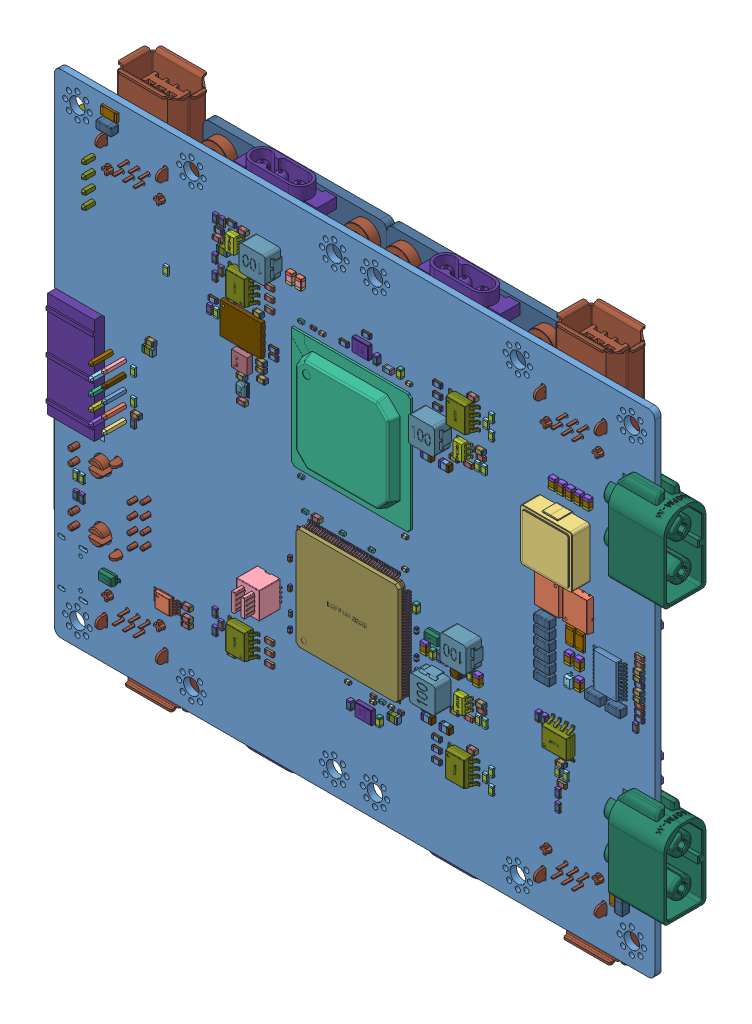
SolidWorks assembly Mother  Board, configuration 默认. Lengths in mm. (continued)
Components (placement in the parent): (continued)
- Mother  Board.step-1: Mother  Board.step [默认] at origin size (122.6 102.08 21) (continued)
  - Free-Models.step-1: Free-Models.step [默认] at origin size (70.87 98.07 8.62) (continued)
    - Driver_Board.step-3: Driver_Board.step [默认] at (57.3933 0 -6.2) x (1 0 0) z (0 0 1) size (35.43 49.03 8.62) (continued)
      - CP4-1.step-1: CP4-1.step [默认] at origin size (1.5 3 1.5)
        - (______)-94.step-1: (______)-94.step [默认] at (7.4932 17.145 0) x (1 0 0) z (0 0 1) size (1.5 3 1.5)
      - CP3-1.step-1: CP3-1.step [默认] at origin size (1.5 3 1.5)
        - (______)-94.step-1: (______)-94.step [默认] at (27.3051 17.1449 0) x (1 0 0) z (0 0 1) size (1.5 3 1.5)
      - CP2-1.step-1: CP2-1.step [默认] at origin size (1.5 3 1.5)
        - (______)-94.step-1: (______)-94.step [默认] at (16.3831 19.4309 0) x (1 0 0) z (0 0 1) size (1.5 3 1.5)
      - CP1-1.step-1: CP1-1.step [默认] at origin size (1.5 3 1.5)
        - (______)-94.step-1: (______)-94.step [默认] at (5.5882 17.145 0) x (1 0 0) z (0 0 1) size (1.5 3 1.5)
      - C29-1.step-1: C29-1.step [默认] at origin size (1.6 0.8 0.8)
        - 6547515616.step-1: 6547515616.step [默认] at (22.9869 16.6369 0) x (-1 0 0) z (0 0 1) size (1.6 0.8 0.8)
          - Terminal-22.step-1: Terminal-22.step [默认] at (-0.8 -0.4 0) size (1.6 0.8 0.8)
            - Open_CASCADE_STEP_translator_6.8_47.1.1-85.step-1: Open_CASCADE_STEP_translator_6.8_47.1.1-85.step [默认] at origin size (0.3 0.8 0.8)
            - Open_CASCADE_STEP_translator_6.8_47.1.2-86.step-1: Open_CASCADE_STEP_translator_6.8_47.1.2-86.step [默认] at origin size (0.3 0.8 0.8)
          - Mid_Body-10.step-1: Mid_Body-10.step [默认] at (-0.8 -0.4 0) size (1 0.8 0.8)
            - Open_CASCADE_STEP_translator_6.8_47.2.1-87.step-1: Open_CASCADE_STEP_translator_6.8_47.2.1-87.step [默认] at origin size (1 0.8 0.8)
      - C28-1.step-1: C28-1.step [默认] at origin size (1.6 0.8 0.8)
        - 6547515616.step-1: 6547515616.step [默认] at (24.6379 10.6679 0) x (-1 0 0) z (0 0 1) size (1.6 0.8 0.8)
          - Terminal-22.step-1: Terminal-22.step [默认] at (-0.8 -0.4 0) size (1.6 0.8 0.8)
            - Open_CASCADE_STEP_translator_6.8_47.1.1-85.step-1: Open_CASCADE_STEP_translator_6.8_47.1.1-85.step [默认] at origin size (0.3 0.8 0.8)
            - Open_CASCADE_STEP_translator_6.8_47.1.2-86.step-1: Open_CASCADE_STEP_translator_6.8_47.1.2-86.step [默认] at origin size (0.3 0.8 0.8)
          - Mid_Body-10.step-1: Mid_Body-10.step [默认] at (-0.8 -0.4 0) size (1 0.8 0.8)
            - Open_CASCADE_STEP_translator_6.8_47.2.1-87.step-1: Open_CASCADE_STEP_translator_6.8_47.2.1-87.step [默认] at origin size (1 0.8 0.8)
      - C27-1.step-1: C27-1.step [默认] at origin size (2.01 1.25 0.94)
        - 6547513136.step-1: 6547513136.step [默认] at (20.8503 23.4725 0) x (-1 0 0) z (0 0 1) size (2.01 1.25 0.94)
          - Fillet1-95.step-1: Fillet1-95.step [默认] at origin size (0.5 1.25 0.94)
          - Fillet2-96.step-1: Fillet2-96.step [默认] at origin size (0.5 1.25 0.94)
          - body2-97.step-1: body2-97.step [默认] at origin size (1.01 1.22 0.92)
      - C26-1.step-1: C26-1.step [默认] at origin size (0.8 1.6 0.8)
        - 6547516096.step-1: 6547516096.step [默认] at (17.9295 24.7425 0) x (0 -1 0) z (0 0 1) size (1.6 0.8 0.8)
          - Terminal-23.step-1: Terminal-23.step [默认] at (-0.8 -0.4 0) size (1.6 0.8 0.8)
            - Open_CASCADE_STEP_translator_6.8_47.1.1-98.step-1: Open_CASCADE_STEP_translator_6.8_47.1.1-98.step [默认] at origin size (0.3 0.8 0.8)
            - Open_CASCADE_STEP_translator_6.8_47.1.2-99.step-1: Open_CASCADE_STEP_translator_6.8_47.1.2-99.step [默认] at origin size (0.3 0.8 0.8)
          - Mid_Body-11.step-1: Mid_Body-11.step [默认] at (-0.8 -0.4 0) size (1 0.8 0.8)
            - Open_CASCADE_STEP_translator_6.8_47.2.1-100.step-1: Open_CASCADE_STEP_translator_6.8_47.2.1-100.step [默认] at origin size (1 0.8 0.8)
      - C25-1.step-1: C25-1.step [默认] at origin size (1.25 2.01 0.94)
        - 6547514896.step-1: 6547514896.step [默认] at (23.5173 31.0126 0) x (0 1 0) z (0 0 1) size (2.01 1.25 0.94)
          - Fillet1-101.step-1: Fillet1-101.step [默认] at origin size (0.5 1.25 0.94)
          - Fillet2-102.step-1: Fillet2-102.step [默认] at origin size (0.5 1.25 0.94)
          - body2-103.step-1: body2-103.step [默认] at origin size (1.01 1.22 0.92)
      - C20-1.step-1: C20-1.step [默认] at origin size (1.6 0.8 0.8)
        - 6547515616.step-1: 6547515616.step [默认] at (12.0649 18.9229 0) x (-1 0 0) z (0 0 1) size (1.6 0.8 0.8)
          - Terminal-22.step-1: Terminal-22.step [默认] at (-0.8 -0.4 0) size (1.6 0.8 0.8)
            - Open_CASCADE_STEP_translator_6.8_47.1.1-85.step-1: Open_CASCADE_STEP_translator_6.8_47.1.1-85.step [默认] at origin size (0.3 0.8 0.8)
            - Open_CASCADE_STEP_translator_6.8_47.1.2-86.step-1: Open_CASCADE_STEP_translator_6.8_47.1.2-86.step [默认] at origin size (0.3 0.8 0.8)
          - Mid_Body-10.step-1: Mid_Body-10.step [默认] at (-0.8 -0.4 0) size (1 0.8 0.8)
            - Open_CASCADE_STEP_translator_6.8_47.2.1-87.step-1: Open_CASCADE_STEP_translator_6.8_47.2.1-87.step [默认] at origin size (1 0.8 0.8)
      - C19-1.step-1: C19-1.step [默认] at origin size (0.8 1.6 0.8)
        - 6547517776.step-1: 6547517776.step [默认] at (25.7809 37.7191 0) x (0 1 0) z (0 0 1) size (1.6 0.8 0.8)
          - Terminal-24.step-1: Terminal-24.step [默认] at (-0.8 -0.4 0) size (1.6 0.8 0.8)
            - Open_CASCADE_STEP_translator_6.8_47.1.1-104.step-1: Open_CASCADE_STEP_translator_6.8_47.1.1-104.step [默认] at origin size (0.3 0.8 0.8)
            - Open_CASCADE_STEP_translator_6.8_47.1.2-105.step-1: Open_CASCADE_STEP_translator_6.8_47.1.2-105.step [默认] at origin size (0.3 0.8 0.8)
          - Mid_Body-12.step-1: Mid_Body-12.step [默认] at (-0.8 -0.4 0) size (1 0.8 0.8)
            - Open_CASCADE_STEP_translator_6.8_47.2.1-106.step-1: Open_CASCADE_STEP_translator_6.8_47.2.1-106.step [默认] at origin size (1 0.8 0.8)
      - C18-1.step-1: C18-1.step [默认] at origin size (0.8 1.6 0.8)
        - 6547517776.step-1: 6547517776.step [默认] at (24.6379 37.7191 0) x (0 1 0) z (0 0 1) size (1.6 0.8 0.8)
          - Terminal-24.step-1: Terminal-24.step [默认] at (-0.8 -0.4 0) size (1.6 0.8 0.8)
            - Open_CASCADE_STEP_translator_6.8_47.1.1-104.step-1: Open_CASCADE_STEP_translator_6.8_47.1.1-104.step [默认] at origin size (0.3 0.8 0.8)
            - Open_CASCADE_STEP_translator_6.8_47.1.2-105.step-1: Open_CASCADE_STEP_translator_6.8_47.1.2-105.step [默认] at origin size (0.3 0.8 0.8)
          - Mid_Body-12.step-1: Mid_Body-12.step [默认] at (-0.8 -0.4 0) size (1 0.8 0.8)
            - Open_CASCADE_STEP_translator_6.8_47.2.1-106.step-1: Open_CASCADE_STEP_translator_6.8_47.2.1-106.step [默认] at origin size (1 0.8 0.8)
      - C17-1.step-1: C17-1.step [默认] at origin size (1.6 0.8 0.8)
        - 6547515616.step-1: 6547515616.step [默认] at (13.7159 12.9539 0) x (-1 0 0) z (0 0 1) size (1.6 0.8 0.8)
          - Terminal-22.step-1: Terminal-22.step [默认] at (-0.8 -0.4 0) size (1.6 0.8 0.8)
            - Open_CASCADE_STEP_translator_6.8_47.1.1-85.step-1: Open_CASCADE_STEP_translator_6.8_47.1.1-85.step [默认] at origin size (0.3 0.8 0.8)
            - Open_CASCADE_STEP_translator_6.8_47.1.2-86.step-1: Open_CASCADE_STEP_translator_6.8_47.1.2-86.step [默认] at origin size (0.3 0.8 0.8)
          - Mid_Body-10.step-1: Mid_Body-10.step [默认] at (-0.8 -0.4 0) size (1 0.8 0.8)
            - Open_CASCADE_STEP_translator_6.8_47.2.1-87.step-1: Open_CASCADE_STEP_translator_6.8_47.2.1-87.step [默认] at origin size (1 0.8 0.8)
      - C16-1.step-1: C16-1.step [默认] at origin size (0.8 1.6 0.8)
        - 6547516096.step-1: 6547516096.step [默认] at (25.7811 22.2249 0) x (0 -1 0) z (0 0 1) size (1.6 0.8 0.8)
          - Terminal-23.step-1: Terminal-23.step [默认] at (-0.8 -0.4 0) size (1.6 0.8 0.8)
            - Open_CASCADE_STEP_translator_6.8_47.1.1-98.step-1: Open_CASCADE_STEP_translator_6.8_47.1.1-98.step [默认] at origin size (0.3 0.8 0.8)
            - Open_CASCADE_STEP_translator_6.8_47.1.2-99.step-1: Open_CASCADE_STEP_translator_6.8_47.1.2-99.step [默认] at origin size (0.3 0.8 0.8)
          - Mid_Body-11.step-1: Mid_Body-11.step [默认] at (-0.8 -0.4 0) size (1 0.8 0.8)
            - Open_CASCADE_STEP_translator_6.8_47.2.1-100.step-1: Open_CASCADE_STEP_translator_6.8_47.2.1-100.step [默认] at origin size (1 0.8 0.8)
      - C15-1.step-1: C15-1.step [默认] at origin size (0.8 1.6 0.8)
        - 6547517776.step-1: 6547517776.step [默认] at (23.8759 25.6541 0) x (0 1 0) z (0 0 1) size (1.6 0.8 0.8)
          - Terminal-24.step-1: Terminal-24.step [默认] at (-0.8 -0.4 0) size (1.6 0.8 0.8)
            - Open_CASCADE_STEP_translator_6.8_47.1.1-104.step-1: Open_CASCADE_STEP_translator_6.8_47.1.1-104.step [默认] at origin size (0.3 0.8 0.8)
            - Open_CASCADE_STEP_translator_6.8_47.1.2-105.step-1: Open_CASCADE_STEP_translator_6.8_47.1.2-105.step [默认] at origin size (0.3 0.8 0.8)
          - Mid_Body-12.step-1: Mid_Body-12.step [默认] at (-0.8 -0.4 0) size (1 0.8 0.8)
            - Open_CASCADE_STEP_translator_6.8_47.2.1-106.step-1: Open_CASCADE_STEP_translator_6.8_47.2.1-106.step [默认] at origin size (1 0.8 0.8)
      - C14-1.step-1: C14-1.step [默认] at origin size (2.01 1.25 0.94)
        - 6547513136.step-1: 6547513136.step [默认] at (13.7383 23.4725 0) x (-1 0 0) z (0 0 1) size (2.01 1.25 0.94)
          - Fillet1-95.step-1: Fillet1-95.step [默认] at origin size (0.5 1.25 0.94)
          - Fillet2-96.step-1: Fillet2-96.step [默认] at origin size (0.5 1.25 0.94)
          - body2-97.step-1: body2-97.step [默认] at origin size (1.01 1.22 0.92)
      - C13-1.step-1: C13-1.step [默认] at origin size (0.8 1.6 0.8)
        - 6547516096.step-1: 6547516096.step [默认] at (10.8175 24.7425 0) x (0 -1 0) z (0 0 1) size (1.6 0.8 0.8)
          - Terminal-23.step-1: Terminal-23.step [默认] at (-0.8 -0.4 0) size (1.6 0.8 0.8)
            - Open_CASCADE_STEP_translator_6.8_47.1.1-98.step-1: Open_CASCADE_STEP_translator_6.8_47.1.1-98.step [默认] at origin size (0.3 0.8 0.8)
            - Open_CASCADE_STEP_translator_6.8_47.1.2-99.step-1: Open_CASCADE_STEP_translator_6.8_47.1.2-99.step [默认] at origin size (0.3 0.8 0.8)
          - Mid_Body-11.step-1: Mid_Body-11.step [默认] at (-0.8 -0.4 0) size (1 0.8 0.8)
            - Open_CASCADE_STEP_translator_6.8_47.2.1-100.step-1: Open_CASCADE_STEP_translator_6.8_47.2.1-100.step [默认] at origin size (1 0.8 0.8)
      - C12-1.step-1: C12-1.step [默认] at origin size (1.25 2.01 0.94)
        - 6547514896.step-1: 6547514896.step [默认] at (16.4053 31.0126 0) x (0 1 0) z (0 0 1) size (2.01 1.25 0.94)
          - Fillet1-101.step-1: Fillet1-101.step [默认] at origin size (0.5 1.25 0.94)
          - Fillet2-102.step-1: Fillet2-102.step [默认] at origin size (0.5 1.25 0.94)
          - body2-103.step-1: body2-103.step [默认] at origin size (1.01 1.22 0.92)
      - C11-1.step-1: C11-1.step [默认] at origin size (1.6 0.8 0.8)
        - 6547515616.step-1: 6547515616.step [默认] at (27.6859 22.8599 0) x (-1 0 0) z (0 0 1) size (1.6 0.8 0.8)
          - Terminal-22.step-1: Terminal-22.step [默认] at (-0.8 -0.4 0) size (1.6 0.8 0.8)
            - Open_CASCADE_STEP_translator_6.8_47.1.1-85.step-1: Open_CASCADE_STEP_translator_6.8_47.1.1-85.step [默认] at origin size (0.3 0.8 0.8)
            - Open_CASCADE_STEP_translator_6.8_47.1.2-86.step-1: Open_CASCADE_STEP_translator_6.8_47.1.2-86.step [默认] at origin size (0.3 0.8 0.8)
          - Mid_Body-10.step-1: Mid_Body-10.step [默认] at (-0.8 -0.4 0) size (1 0.8 0.8)
            - Open_CASCADE_STEP_translator_6.8_47.2.1-87.step-1: Open_CASCADE_STEP_translator_6.8_47.2.1-87.step [默认] at origin size (1 0.8 0.8)
      - C10-1.step-1: C10-1.step [默认] at origin size (0.8 1.6 0.8)
        - 6547517776.step-1: 6547517776.step [默认] at (-3.1751 37.7191 0) x (0 1 0) z (0 0 1) size (1.6 0.8 0.8)
          - Terminal-24.step-1: Terminal-24.step [默认] at (-0.8 -0.4 0) size (1.6 0.8 0.8)
            - Open_CASCADE_STEP_translator_6.8_47.1.1-104.step-1: Open_CASCADE_STEP_translator_6.8_47.1.1-104.step [默认] at origin size (0.3 0.8 0.8)
            - Open_CASCADE_STEP_translator_6.8_47.1.2-105.step-1: Open_CASCADE_STEP_translator_6.8_47.1.2-105.step [默认] at origin size (0.3 0.8 0.8)
          - Mid_Body-12.step-1: Mid_Body-12.step [默认] at (-0.8 -0.4 0) size (1 0.8 0.8)
            - Open_CASCADE_STEP_translator_6.8_47.2.1-106.step-1: Open_CASCADE_STEP_translator_6.8_47.2.1-106.step [默认] at origin size (1 0.8 0.8)
      - C9-1.step-1: C9-1.step [默认] at origin size (0.8 1.6 0.8)
        - 6547516096.step-1: 6547516096.step [默认] at (-3.1749 22.2249 0) x (0 -1 0) z (0 0 1) size (1.6 0.8 0.8)
          - Terminal-23.step-1: Terminal-23.step [默认] at (-0.8 -0.4 0) size (1.6 0.8 0.8)
            - Open_CASCADE_STEP_translator_6.8_47.1.1-98.step-1: Open_CASCADE_STEP_translator_6.8_47.1.1-98.step [默认] at origin size (0.3 0.8 0.8)
            - Open_CASCADE_STEP_translator_6.8_47.1.2-99.step-1: Open_CASCADE_STEP_translator_6.8_47.1.2-99.step [默认] at origin size (0.3 0.8 0.8)
          - Mid_Body-11.step-1: Mid_Body-11.step [默认] at (-0.8 -0.4 0) size (1 0.8 0.8)
            - Open_CASCADE_STEP_translator_6.8_47.2.1-100.step-1: Open_CASCADE_STEP_translator_6.8_47.2.1-100.step [默认] at origin size (1 0.8 0.8)
      - C8-1.step-1: C8-1.step [默认] at origin size (1.6 0.8 0.8)
        - 6547515616.step-1: 6547515616.step [默认] at (1.1429 16.5099 0) x (-1 0 0) z (0 0 1) size (1.6 0.8 0.8)
          - Terminal-22.step-1: Terminal-22.step [默认] at (-0.8 -0.4 0) size (1.6 0.8 0.8)
            - Open_CASCADE_STEP_translator_6.8_47.1.1-85.step-1: Open_CASCADE_STEP_translator_6.8_47.1.1-85.step [默认] at origin size (0.3 0.8 0.8)
            - Open_CASCADE_STEP_translator_6.8_47.1.2-86.step-1: Open_CASCADE_STEP_translator_6.8_47.1.2-86.step [默认] at origin size (0.3 0.8 0.8)
          - Mid_Body-10.step-1: Mid_Body-10.step [默认] at (-0.8 -0.4 0) size (1 0.8 0.8)
            - Open_CASCADE_STEP_translator_6.8_47.2.1-87.step-1: Open_CASCADE_STEP_translator_6.8_47.2.1-87.step [默认] at origin size (1 0.8 0.8)
      - C7-1.step-1: C7-1.step [默认] at origin size (0.8 1.6 0.8)
        - 6547516096.step-1: 6547516096.step [默认] at (-2.0319 22.2249 0) x (0 -1 0) z (0 0 1) size (1.6 0.8 0.8)
          - Terminal-23.step-1: Terminal-23.step [默认] at (-0.8 -0.4 0) size (1.6 0.8 0.8)
            - Open_CASCADE_STEP_translator_6.8_47.1.1-98.step-1: Open_CASCADE_STEP_translator_6.8_47.1.1-98.step [默认] at origin size (0.3 0.8 0.8)
            - Open_CASCADE_STEP_translator_6.8_47.1.2-99.step-1: Open_CASCADE_STEP_translator_6.8_47.1.2-99.step [默认] at origin size (0.3 0.8 0.8)
          - Mid_Body-11.step-1: Mid_Body-11.step [默认] at (-0.8 -0.4 0) size (1 0.8 0.8)
            - Open_CASCADE_STEP_translator_6.8_47.2.1-100.step-1: Open_CASCADE_STEP_translator_6.8_47.2.1-100.step [默认] at origin size (1 0.8 0.8)
      - C6-1.step-1: C6-1.step [默认] at origin size (0.8 1.6 0.8)
        - 6547517776.step-1: 6547517776.step [默认] at (-2.0321 37.7191 0) x (0 1 0) z (0 0 1) size (1.6 0.8 0.8)
          - Terminal-24.step-1: Terminal-24.step [默认] at (-0.8 -0.4 0) size (1.6 0.8 0.8)
            - Open_CASCADE_STEP_translator_6.8_47.1.1-104.step-1: Open_CASCADE_STEP_translator_6.8_47.1.1-104.step [默认] at origin size (0.3 0.8 0.8)
            - Open_CASCADE_STEP_translator_6.8_47.1.2-105.step-1: Open_CASCADE_STEP_translator_6.8_47.1.2-105.step [默认] at origin size (0.3 0.8 0.8)
          - Mid_Body-12.step-1: Mid_Body-12.step [默认] at (-0.8 -0.4 0) size (1 0.8 0.8)
            - Open_CASCADE_STEP_translator_6.8_47.2.1-106.step-1: Open_CASCADE_STEP_translator_6.8_47.2.1-106.step [默认] at origin size (1 0.8 0.8)
      - C5-1.step-1: C5-1.step [默认] at origin size (1.6 0.8 0.8)
        - 6547515616.step-1: 6547515616.step [默认] at (2.7939 10.6679 0) x (-1 0 0) z (0 0 1) size (1.6 0.8 0.8)
          - Terminal-22.step-1: Terminal-22.step [默认] at (-0.8 -0.4 0) size (1.6 0.8 0.8)
            - Open_CASCADE_STEP_translator_6.8_47.1.1-85.step-1: Open_CASCADE_STEP_translator_6.8_47.1.1-85.step [默认] at origin size (0.3 0.8 0.8)
            - Open_CASCADE_STEP_translator_6.8_47.1.2-86.step-1: Open_CASCADE_STEP_translator_6.8_47.1.2-86.step [默认] at origin size (0.3 0.8 0.8)
          - Mid_Body-10.step-1: Mid_Body-10.step [默认] at (-0.8 -0.4 0) size (1 0.8 0.8)
            - Open_CASCADE_STEP_translator_6.8_47.2.1-87.step-1: Open_CASCADE_STEP_translator_6.8_47.2.1-87.step [默认] at origin size (1 0.8 0.8)
      - C4-1.step-1: C4-1.step [默认] at origin size (1.6 0.8 0.8)
        - 6547515616.step-1: 6547515616.step [默认] at (-0.1271 22.8599 0) x (-1 0 0) z (0 0 1) size (1.6 0.8 0.8)
          - Terminal-22.step-1: Terminal-22.step [默认] at (-0.8 -0.4 0) size (1.6 0.8 0.8)
            - Open_CASCADE_STEP_translator_6.8_47.1.1-85.step-1: Open_CASCADE_STEP_translator_6.8_47.1.1-85.step [默认] at origin size (0.3 0.8 0.8)
            - Open_CASCADE_STEP_translator_6.8_47.1.2-86.step-1: Open_CASCADE_STEP_translator_6.8_47.1.2-86.step [默认] at origin size (0.3 0.8 0.8)
          - Mid_Body-10.step-1: Mid_Body-10.step [默认] at (-0.8 -0.4 0) size (1 0.8 0.8)
            - Open_CASCADE_STEP_translator_6.8_47.2.1-87.step-1: Open_CASCADE_STEP_translator_6.8_47.2.1-87.step [默认] at origin size (1 0.8 0.8)
      - C3-1.step-1: C3-1.step [默认] at origin size (2.01 1.25 0.94)
        - 6547513136.step-1: 6547513136.step [默认] at (6.6263 23.4725 0) x (-1 0 0) z (0 0 1) size (2.01 1.25 0.94)
          - Fillet1-95.step-1: Fillet1-95.step [默认] at origin size (0.5 1.25 0.94)
          - Fillet2-96.step-1: Fillet2-96.step [默认] at origin size (0.5 1.25 0.94)
          - body2-97.step-1: body2-97.step [默认] at origin size (1.01 1.22 0.92)
      - C2-1.step-1: C2-1.step [默认] at origin size (0.8 1.6 0.8)
        - 6547516096.step-1: 6547516096.step [默认] at (3.7055 24.7425 0) x (0 -1 0) z (0 0 1) size (1.6 0.8 0.8)
          - Terminal-23.step-1: Terminal-23.step [默认] at (-0.8 -0.4 0) size (1.6 0.8 0.8)
            - Open_CASCADE_STEP_translator_6.8_47.1.1-98.step-1: Open_CASCADE_STEP_translator_6.8_47.1.1-98.step [默认] at origin size (0.3 0.8 0.8)
            - Open_CASCADE_STEP_translator_6.8_47.1.2-99.step-1: Open_CASCADE_STEP_translator_6.8_47.1.2-99.step [默认] at origin size (0.3 0.8 0.8)
          - Mid_Body-11.step-1: Mid_Body-11.step [默认] at (-0.8 -0.4 0) size (1 0.8 0.8)
            - Open_CASCADE_STEP_translator_6.8_47.2.1-100.step-1: Open_CASCADE_STEP_translator_6.8_47.2.1-100.step [默认] at origin size (1 0.8 0.8)
      - C1.step-1: C1.step [默认] at origin size (1.25 2.01 0.94)
        - 6547514896.step-1: 6547514896.step [默认] at (9.2933 31.0126 0) x (0 1 0) z (0 0 1) size (2.01 1.25 0.94)
          - Fillet1-101.step-1: Fillet1-101.step [默认] at origin size (0.5 1.25 0.94)
          - Fillet2-102.step-1: Fillet2-102.step [默认] at origin size (0.5 1.25 0.94)
          - body2-103.step-1: body2-103.step [默认] at origin size (1.01 1.22 0.92)
    - Driver_Board.step-4: Driver_Board.step [默认] at (21.971 0 -6.2) x (1 0 0) z (0 0 1) size (35.43 49.03 8.62)
      - Board-1.step-1: Board-1.step [默认] at origin size (35.43 46.99 1.62)
        - Open_CASCADE_STEP_translator_6.8_2.1.1.step-1: Open_CASCADE_STEP_translator_6.8_2.1.1.step [默认] at (0 0 -1.6164) size (35.43 46.99 1.62)
      - R25-1.step-1: R25-1.step [默认] at origin size (0.8 1.6 0.45)
        - 6547515376.step-1: 6547515376.step [默认] at (20.6304 35.5601 0) x (0 1 0) z (0 0 1) size (1.6 0.8 0.45)
          - Terminal-19.step-1: Terminal-19.step [默认] at (-0.8 -0.4 0) size (0.3 0.8 0.45)
            - Open_CASCADE_STEP_translator_6.8_21.2.1-76.step-1: Open_CASCADE_STEP_translator_6.8_21.2.1-76.step [默认] at origin size (0.3 0.8 0.45)
          - Terminal-19.step-2: Terminal-19.step [默认] at (0.8 0.4 0) x (-1 0 0) z (0 0 1) size (0.3 0.8 0.45)
            - Open_CASCADE_STEP_translator_6.8_21.2.1-76.step-1: Open_CASCADE_STEP_translator_6.8_21.2.1-76.step [默认] at origin size (0.3 0.8 0.45)
          - Mid_Body-77.step-1: Mid_Body-77.step [默认] at (-0.8 -0.4 0) size (1.51 0.8 0.36)
          - Mark-78.step-1: Mark-78.step [默认] at (-0.5 -0.4 0.405) size (1 0.8 0.05)
      - R24-1.step-1: R24-1.step [默认] at origin size (1.6 0.8 0.45)
        - 6547516336.step-1: 6547516336.step [默认] at (12.6999 34.9249 0) x (-1 0 0) z (0 0 1) size (1.6 0.8 0.45)
          - Terminal-20.step-1: Terminal-20.step [默认] at (-0.8 -0.4 0) size (0.3 0.8 0.45)
            - Open_CASCADE_STEP_translator_6.8_21.2.1-79.step-1: Open_CASCADE_STEP_translator_6.8_21.2.1-79.step [默认] at origin size (0.3 0.8 0.45)
          - Terminal-20.step-2: Terminal-20.step [默认] at (0.8 0.4 0) x (-1 0 0) z (0 0 1) size (0.3 0.8 0.45)
            - Open_CASCADE_STEP_translator_6.8_21.2.1-79.step-1: Open_CASCADE_STEP_translator_6.8_21.2.1-79.step [默认] at origin size (0.3 0.8 0.45)
          - Mid_Body-80.step-1: Mid_Body-80.step [默认] at (-0.8 -0.4 0) size (1.51 0.8 0.36)
          - Mark-81.step-1: Mark-81.step [默认] at (-0.5 -0.4 0.405) size (1 0.8 0.05)
      - R23-1.step-1: R23-1.step [默认] at origin size (1.6 0.8 0.45)
        - 6547516336.step-1: 6547516336.step [默认] at (5.5879 33.6549 0) x (-1 0 0) z (0 0 1) size (1.6 0.8 0.45)
          - Terminal-20.step-1: Terminal-20.step [默认] at (-0.8 -0.4 0) size (0.3 0.8 0.45)
            - Open_CASCADE_STEP_translator_6.8_21.2.1-79.step-1: Open_CASCADE_STEP_translator_6.8_21.2.1-79.step [默认] at origin size (0.3 0.8 0.45)
          - Terminal-20.step-2: Terminal-20.step [默认] at (0.8 0.4 0) x (-1 0 0) z (0 0 1) size (0.3 0.8 0.45)
            - Open_CASCADE_STEP_translator_6.8_21.2.1-79.step-1: Open_CASCADE_STEP_translator_6.8_21.2.1-79.step [默认] at origin size (0.3 0.8 0.45)
          - Mid_Body-80.step-1: Mid_Body-80.step [默认] at (-0.8 -0.4 0) size (1.51 0.8 0.36)
          - Mark-81.step-1: Mark-81.step [默认] at (-0.5 -0.4 0.405) size (1 0.8 0.05)
      - JP1.step-1: JP1.step [默认] at origin size (16.01 14.49 6.96)
        - User_Library-MR30PW-M.step-1: User_Library-MR30PW-M.step [默认] at (13.7158 -5.9802 2.75) x (1 0 0) z (0 0 1) size (16.01 14.49 6.96)
      - R18-1.step-1: R18-1.step [默认] at origin size (0.8 1.6 0.45)
        - 6547515376.step-1: 6547515376.step [默认] at (22.9869 34.4171 0) x (0 1 0) z (0 0 1) size (1.6 0.8 0.45)
          - Terminal-19.step-1: Terminal-19.step [默认] at (-0.8 -0.4 0) size (0.3 0.8 0.45)
            - Open_CASCADE_STEP_translator_6.8_21.2.1-76.step-1: Open_CASCADE_STEP_translator_6.8_21.2.1-76.step [默认] at origin size (0.3 0.8 0.45)
          - Terminal-19.step-2: Terminal-19.step [默认] at (0.8 0.4 0) x (-1 0 0) z (0 0 1) size (0.3 0.8 0.45)
            - Open_CASCADE_STEP_translator_6.8_21.2.1-76.step-1: Open_CASCADE_STEP_translator_6.8_21.2.1-76.step [默认] at origin size (0.3 0.8 0.45)
          - Mid_Body-77.step-1: Mid_Body-77.step [默认] at (-0.8 -0.4 0) size (1.51 0.8 0.36)
          - Mark-78.step-1: Mark-78.step [默认] at (-0.5 -0.4 0.405) size (1 0.8 0.05)
      - R17-1.step-1: R17-1.step [默认] at origin size (0.8 1.6 0.45)
        - 6547515376.step-1: 6547515376.step [默认] at (21.8663 34.3947 0) x (0 1 0) z (0 0 1) size (1.6 0.8 0.45)
          - Terminal-19.step-1: Terminal-19.step [默认] at (-0.8 -0.4 0) size (0.3 0.8 0.45)
            - Open_CASCADE_STEP_translator_6.8_21.2.1-76.step-1: Open_CASCADE_STEP_translator_6.8_21.2.1-76.step [默认] at origin size (0.3 0.8 0.45)
          - Terminal-19.step-2: Terminal-19.step [默认] at (0.8 0.4 0) x (-1 0 0) z (0 0 1) size (0.3 0.8 0.45)
            - Open_CASCADE_STEP_translator_6.8_21.2.1-76.step-1: Open_CASCADE_STEP_translator_6.8_21.2.1-76.step [默认] at origin size (0.3 0.8 0.45)
          - Mid_Body-77.step-1: Mid_Body-77.step [默认] at (-0.8 -0.4 0) size (1.51 0.8 0.36)
          - Mark-78.step-1: Mark-78.step [默认] at (-0.5 -0.4 0.405) size (1 0.8 0.05)
      - R16-1.step-1: R16-1.step [默认] at origin size (1.6 0.8 0.45)
        - 6547506496.step-1: 6547506496.step [默认] at (16.6371 33.6551 0) x (1 0 0) z (0 0 1) size (1.6 0.8 0.45)
          - Terminal-21.step-1: Terminal-21.step [默认] at (-0.8 -0.4 0) size (0.3 0.8 0.45)
            - Open_CASCADE_STEP_translator_6.8_21.2.1-82.step-1: Open_CASCADE_STEP_translator_6.8_21.2.1-82.step [默认] at origin size (0.3 0.8 0.45)
          - Terminal-21.step-2: Terminal-21.step [默认] at (0.8 0.4 0) x (-1 0 0) z (0 0 1) size (0.3 0.8 0.45)
            - Open_CASCADE_STEP_translator_6.8_21.2.1-82.step-1: Open_CASCADE_STEP_translator_6.8_21.2.1-82.step [默认] at origin size (0.3 0.8 0.45)
          - Mid_Body-83.step-1: Mid_Body-83.step [默认] at (-0.8 -0.4 0) size (1.51 0.8 0.36)
          - Mark-84.step-1: Mark-84.step [默认] at (-0.5 -0.4 0.405) size (1 0.8 0.05)
      - R15-1.step-1: R15-1.step [默认] at origin size (0.8 1.6 0.45)
        - 6547515376.step-1: 6547515376.step [默认] at (14.7319 34.2901 0) x (0 1 0) z (0 0 1) size (1.6 0.8 0.45)
          - Terminal-19.step-1: Terminal-19.step [默认] at (-0.8 -0.4 0) size (0.3 0.8 0.45)
            - Open_CASCADE_STEP_translator_6.8_21.2.1-76.step-1: Open_CASCADE_STEP_translator_6.8_21.2.1-76.step [默认] at origin size (0.3 0.8 0.45)
          - Terminal-19.step-2: Terminal-19.step [默认] at (0.8 0.4 0) x (-1 0 0) z (0 0 1) size (0.3 0.8 0.45)
            - Open_CASCADE_STEP_translator_6.8_21.2.1-76.step-1: Open_CASCADE_STEP_translator_6.8_21.2.1-76.step [默认] at origin size (0.3 0.8 0.45)
          - Mid_Body-77.step-1: Mid_Body-77.step [默认] at (-0.8 -0.4 0) size (1.51 0.8 0.36)
          - Mark-78.step-1: Mark-78.step [默认] at (-0.5 -0.4 0.405) size (1 0.8 0.05)
      - R13-1.step-1: R13-1.step [默认] at origin size (1.6 0.8 0.45)
        - 6547506496.step-1: 6547506496.step [默认] at (9.5251 33.6551 0) x (1 0 0) z (0 0 1) size (1.6 0.8 0.45)
          - Terminal-21.step-1: Terminal-21.step [默认] at (-0.8 -0.4 0) size (0.3 0.8 0.45)
            - Open_CASCADE_STEP_translator_6.8_21.2.1-82.step-1: Open_CASCADE_STEP_translator_6.8_21.2.1-82.step [默认] at origin size (0.3 0.8 0.45)
          - Terminal-21.step-2: Terminal-21.step [默认] at (0.8 0.4 0) x (-1 0 0) z (0 0 1) size (0.3 0.8 0.45)
            - Open_CASCADE_STEP_translator_6.8_21.2.1-82.step-1: Open_CASCADE_STEP_translator_6.8_21.2.1-82.step [默认] at origin size (0.3 0.8 0.45)
          - Mid_Body-83.step-1: Mid_Body-83.step [默认] at (-0.8 -0.4 0) size (1.51 0.8 0.36)
          - Mark-84.step-1: Mark-84.step [默认] at (-0.5 -0.4 0.405) size (1 0.8 0.05)
      - R11-1.step-1: R11-1.step [默认] at origin size (0.8 1.6 0.45)
        - 6547515376.step-1: 6547515376.step [默认] at (7.6423 34.2901 0) x (0 1 0) z (0 0 1) size (1.6 0.8 0.45)
          - Terminal-19.step-1: Terminal-19.step [默认] at (-0.8 -0.4 0) size (0.3 0.8 0.45)
            - Open_CASCADE_STEP_translator_6.8_21.2.1-76.step-1: Open_CASCADE_STEP_translator_6.8_21.2.1-76.step [默认] at origin size (0.3 0.8 0.45)
          - Terminal-19.step-2: Terminal-19.step [默认] at (0.8 0.4 0) x (-1 0 0) z (0 0 1) size (0.3 0.8 0.45)
            - Open_CASCADE_STEP_translator_6.8_21.2.1-76.step-1: Open_CASCADE_STEP_translator_6.8_21.2.1-76.step [默认] at origin size (0.3 0.8 0.45)
          - Mid_Body-77.step-1: Mid_Body-77.step [默认] at (-0.8 -0.4 0) size (1.51 0.8 0.36)
          - Mark-78.step-1: Mark-78.step [默认] at (-0.5 -0.4 0.405) size (1 0.8 0.05)
      - C23-1.step-1: C23-1.step [默认] at origin size (1.6 0.8 0.8)
        - 6547515616.step-1: 6547515616.step [默认] at (19.8684 33.6676 0) x (-1 0 0) z (0 0 1) size (1.6 0.8 0.8)
          - Terminal-22.step-1: Terminal-22.step [默认] at (-0.8 -0.4 0) size (1.6 0.8 0.8)
            - Open_CASCADE_STEP_translator_6.8_47.1.1-85.step-1: Open_CASCADE_STEP_translator_6.8_47.1.1-85.step [默认] at origin size (0.3 0.8 0.8)
            - Open_CASCADE_STEP_translator_6.8_47.1.2-86.step-1: Open_CASCADE_STEP_translator_6.8_47.1.2-86.step [默认] at origin size (0.3 0.8 0.8)
          - Mid_Body-10.step-1: Mid_Body-10.step [默认] at (-0.8 -0.4 0) size (1 0.8 0.8)
            - Open_CASCADE_STEP_translator_6.8_47.2.1-87.step-1: Open_CASCADE_STEP_translator_6.8_47.2.1-87.step [默认] at origin size (1 0.8 0.8)
      - C22-1.step-1: C22-1.step [默认] at origin size (1.6 0.8 0.8)
        - 6547515616.step-1: 6547515616.step [默认] at (12.6999 33.6549 0) x (-1 0 0) z (0 0 1) size (1.6 0.8 0.8)
          - Terminal-22.step-1: Terminal-22.step [默认] at (-0.8 -0.4 0) size (1.6 0.8 0.8)
            - Open_CASCADE_STEP_translator_6.8_47.1.1-85.step-1: Open_CASCADE_STEP_translator_6.8_47.1.1-85.step [默认] at origin size (0.3 0.8 0.8)
            - Open_CASCADE_STEP_translator_6.8_47.1.2-86.step-1: Open_CASCADE_STEP_translator_6.8_47.1.2-86.step [默认] at origin size (0.3 0.8 0.8)
          - Mid_Body-10.step-1: Mid_Body-10.step [默认] at (-0.8 -0.4 0) size (1 0.8 0.8)
            - Open_CASCADE_STEP_translator_6.8_47.2.1-87.step-1: Open_CASCADE_STEP_translator_6.8_47.2.1-87.step [默认] at origin size (1 0.8 0.8)
      - C21-1.step-1: C21-1.step [默认] at origin size (1.6 0.8 0.8)
        - 6547515616.step-1: 6547515616.step [默认] at (5.6103 34.9025 0) x (-1 0 0) z (0 0 1) size (1.6 0.8 0.8)
          - Terminal-22.step-1: Terminal-22.step [默认] at (-0.8 -0.4 0) size (1.6 0.8 0.8)
            - Open_CASCADE_STEP_translator_6.8_47.1.1-85.step-1: Open_CASCADE_STEP_translator_6.8_47.1.1-85.step [默认] at origin size (0.3 0.8 0.8)
            - Open_CASCADE_STEP_translator_6.8_47.1.2-86.step-1: Open_CASCADE_STEP_translator_6.8_47.1.2-86.step [默认] at origin size (0.3 0.8 0.8)
          - Mid_Body-10.step-1: Mid_Body-10.step [默认] at (-0.8 -0.4 0) size (1 0.8 0.8)
            - Open_CASCADE_STEP_translator_6.8_47.2.1-87.step-1: Open_CASCADE_STEP_translator_6.8_47.2.1-87.step [默认] at origin size (1 0.8 0.8)
      - U5-1.step-1: U5-1.step [默认] at origin size (5.9 11.5 2.7)
        - SO8_W.step-1: SO8_W.step [默认] at (27.6859 29.9721 0.381) x (0 1 0) z (0 0 1) size (11.5 5.9 2.7)
      - U4-1.step-1: U4-1.step [默认] at origin size (5.9 11.5 2.7)
        - SO8_W.step-1: SO8_W.step [默认] at (-0.1271 29.9721 0.381) x (0 1 0) z (0 0 1) size (11.5 5.9 2.7)
      - U3-1.step-1: U3-1.step [默认] at origin size (5 6.01 1.9)
        - SOP8-1.step-1: SOP8-1.step [默认] at (19.9615 29.5285 0) x (0 -1 0) z (0 0 1) size (6.01 5 1.9)
          - LOGO_-88.step-1: LOGO_-88.step [默认] at (0.0116 0 0.095) x (0 -1 0) z (0 0 -1) size (1.5 1.73 0.01)
          - SOP8-89.step-1: SOP8-89.step [默认] at origin size (6.01 5 1.9)
      - U2-1.step-1: U2-1.step [默认] at origin size (5 6.01 1.9)
        - SOP8-1.step-1: SOP8-1.step [默认] at (12.8495 29.5285 0) x (0 -1 0) z (0 0 1) size (6.01 5 1.9)
          - LOGO_-88.step-1: LOGO_-88.step [默认] at (0.0116 0 0.095) x (0 -1 0) z (0 0 -1) size (1.5 1.73 0.01)
          - SOP8-89.step-1: SOP8-89.step [默认] at origin size (6.01 5 1.9)
      - U1.step-1: U1.step [默认] at origin size (5 6.01 1.9)
        - SOP8-1.step-1: SOP8-1.step [默认] at (5.7375 29.5285 0) x (0 -1 0) z (0 0 1) size (6.01 5 1.9)
          - LOGO_-88.step-1: LOGO_-88.step [默认] at (0.0116 0 0.095) x (0 -1 0) z (0 0 -1) size (1.5 1.73 0.01)
          - SOP8-89.step-1: SOP8-89.step [默认] at origin size (6.01 5 1.9)
      - RS2-1.step-1: RS2-1.step [默认] at origin size (3.1 1.55 0.47)
        - User_Library-R1206-90.step-1: User_Library-R1206-90.step [默认] at (23.7489 17.5261 -1.6164) x (-1 0 0) z (0 0 -1) size (3.1 1.55 0.47)
      - RS1-1.step-1: RS1-1.step [默认] at origin size (3.1 1.55 0.47)
        - User_Library-R1206-90.step-1: User_Library-R1206-90.step [默认] at (-0.1271 18.1611 -1.6164) x (-1 0 0) z (0 0 -1) size (3.1 1.55 0.47)
      - R22-1.step-1: R22-1.step [默认] at origin size (1.6 0.8 0.45)
        - 6547506496.step-1: 6547506496.step [默认] at (22.9871 17.7801 0) x (1 0 0) z (0 0 1) size (1.6 0.8 0.45)
          - Terminal-21.step-1: Terminal-21.step [默认] at (-0.8 -0.4 0) size (0.3 0.8 0.45)
            - Open_CASCADE_STEP_translator_6.8_21.2.1-82.step-1: Open_CASCADE_STEP_translator_6.8_21.2.1-82.step [默认] at origin size (0.3 0.8 0.45)
          - Terminal-21.step-2: Terminal-21.step [默认] at (0.8 0.4 0) x (-1 0 0) z (0 0 1) size (0.3 0.8 0.45)
            - Open_CASCADE_STEP_translator_6.8_21.2.1-82.step-1: Open_CASCADE_STEP_translator_6.8_21.2.1-82.step [默认] at origin size (0.3 0.8 0.45)
          - Mid_Body-83.step-1: Mid_Body-83.step [默认] at (-0.8 -0.4 0) size (1.51 0.8 0.36)
          - Mark-84.step-1: Mark-84.step [默认] at (-0.5 -0.4 0.405) size (1 0.8 0.05)
      - R21-1.step-1: R21-1.step [默认] at origin size (1.6 0.8 0.45)
        - 6547516336.step-1: 6547516336.step [默认] at (22.9869 18.9229 0) x (-1 0 0) z (0 0 1) size (1.6 0.8 0.45)
          - Terminal-20.step-1: Terminal-20.step [默认] at (-0.8 -0.4 0) size (0.3 0.8 0.45)
            - Open_CASCADE_STEP_translator_6.8_21.2.1-79.step-1: Open_CASCADE_STEP_translator_6.8_21.2.1-79.step [默认] at origin size (0.3 0.8 0.45)
          - Terminal-20.step-2: Terminal-20.step [默认] at (0.8 0.4 0) x (-1 0 0) z (0 0 1) size (0.3 0.8 0.45)
            - Open_CASCADE_STEP_translator_6.8_21.2.1-79.step-1: Open_CASCADE_STEP_translator_6.8_21.2.1-79.step [默认] at origin size (0.3 0.8 0.45)
          - Mid_Body-80.step-1: Mid_Body-80.step [默认] at (-0.8 -0.4 0) size (1.51 0.8 0.36)
          - Mark-81.step-1: Mark-81.step [默认] at (-0.5 -0.4 0.405) size (1 0.8 0.05)
      - R20-1.step-1: R20-1.step [默认] at origin size (1.6 0.8 0.45)
        - 6547506496.step-1: 6547506496.step [默认] at (24.6381 11.8111 0) x (1 0 0) z (0 0 1) size (1.6 0.8 0.45)
          - Terminal-21.step-1: Terminal-21.step [默认] at (-0.8 -0.4 0) size (0.3 0.8 0.45)
            - Open_CASCADE_STEP_translator_6.8_21.2.1-82.step-1: Open_CASCADE_STEP_translator_6.8_21.2.1-82.step [默认] at origin size (0.3 0.8 0.45)
          - Terminal-21.step-2: Terminal-21.step [默认] at (0.8 0.4 0) x (-1 0 0) z (0 0 1) size (0.3 0.8 0.45)
            - Open_CASCADE_STEP_translator_6.8_21.2.1-82.step-1: Open_CASCADE_STEP_translator_6.8_21.2.1-82.step [默认] at origin size (0.3 0.8 0.45)
          - Mid_Body-83.step-1: Mid_Body-83.step [默认] at (-0.8 -0.4 0) size (1.51 0.8 0.36)
          - Mark-84.step-1: Mark-84.step [默认] at (-0.5 -0.4 0.405) size (1 0.8 0.05)
      - R19-1.step-1: R19-1.step [默认] at origin size (0.8 1.6 0.45)
        - 6547515376.step-1: 6547515376.step [默认] at (25.3999 13.5891 0) x (0 1 0) z (0 0 1) size (1.6 0.8 0.45)
          - Terminal-19.step-1: Terminal-19.step [默认] at (-0.8 -0.4 0) size (0.3 0.8 0.45)
            - Open_CASCADE_STEP_translator_6.8_21.2.1-76.step-1: Open_CASCADE_STEP_translator_6.8_21.2.1-76.step [默认] at origin size (0.3 0.8 0.45)
          - Terminal-19.step-2: Terminal-19.step [默认] at (0.8 0.4 0) x (-1 0 0) z (0 0 1) size (0.3 0.8 0.45)
            - Open_CASCADE_STEP_translator_6.8_21.2.1-76.step-1: Open_CASCADE_STEP_translator_6.8_21.2.1-76.step [默认] at origin size (0.3 0.8 0.45)
          - Mid_Body-77.step-1: Mid_Body-77.step [默认] at (-0.8 -0.4 0) size (1.51 0.8 0.36)
          - Mark-78.step-1: Mark-78.step [默认] at (-0.5 -0.4 0.405) size (1 0.8 0.05)
      - R14-1.step-1: R14-1.step [默认] at origin size (1.6 0.8 0.45)
        - 6547506496.step-1: 6547506496.step [默认] at (12.0651 20.0661 0) x (1 0 0) z (0 0 1) size (1.6 0.8 0.45)
          - Terminal-21.step-1: Terminal-21.step [默认] at (-0.8 -0.4 0) size (0.3 0.8 0.45)
            - Open_CASCADE_STEP_translator_6.8_21.2.1-82.step-1: Open_CASCADE_STEP_translator_6.8_21.2.1-82.step [默认] at origin size (0.3 0.8 0.45)
          - Terminal-21.step-2: Terminal-21.step [默认] at (0.8 0.4 0) x (-1 0 0) z (0 0 1) size (0.3 0.8 0.45)
            - Open_CASCADE_STEP_translator_6.8_21.2.1-82.step-1: Open_CASCADE_STEP_translator_6.8_21.2.1-82.step [默认] at origin size (0.3 0.8 0.45)
          - Mid_Body-83.step-1: Mid_Body-83.step [默认] at (-0.8 -0.4 0) size (1.51 0.8 0.36)
          - Mark-84.step-1: Mark-84.step [默认] at (-0.5 -0.4 0.405) size (1 0.8 0.05)
      - R12-1.step-1: R12-1.step [默认] at origin size (1.6 0.8 0.45)
        - 6547516336.step-1: 6547516336.step [默认] at (12.0649 21.2089 0) x (-1 0 0) z (0 0 1) size (1.6 0.8 0.45)
          - Terminal-20.step-1: Terminal-20.step [默认] at (-0.8 -0.4 0) size (0.3 0.8 0.45)
            - Open_CASCADE_STEP_translator_6.8_21.2.1-79.step-1: Open_CASCADE_STEP_translator_6.8_21.2.1-79.step [默认] at origin size (0.3 0.8 0.45)
          - Terminal-20.step-2: Terminal-20.step [默认] at (0.8 0.4 0) x (-1 0 0) z (0 0 1) size (0.3 0.8 0.45)
            - Open_CASCADE_STEP_translator_6.8_21.2.1-79.step-1: Open_CASCADE_STEP_translator_6.8_21.2.1-79.step [默认] at origin size (0.3 0.8 0.45)
          - Mid_Body-80.step-1: Mid_Body-80.step [默认] at (-0.8 -0.4 0) size (1.51 0.8 0.36)
          - Mark-81.step-1: Mark-81.step [默认] at (-0.5 -0.4 0.405) size (1 0.8 0.05)
      - R10-1.step-1: R10-1.step [默认] at origin size (1.6 0.8 0.45)
        - 6547506496.step-1: 6547506496.step [默认] at (13.7161 14.0971 0) x (1 0 0) z (0 0 1) size (1.6 0.8 0.45)
          - Terminal-21.step-1: Terminal-21.step [默认] at (-0.8 -0.4 0) size (0.3 0.8 0.45)
            - Open_CASCADE_STEP_translator_6.8_21.2.1-82.step-1: Open_CASCADE_STEP_translator_6.8_21.2.1-82.step [默认] at origin size (0.3 0.8 0.45)
          - Terminal-21.step-2: Terminal-21.step [默认] at (0.8 0.4 0) x (-1 0 0) z (0 0 1) size (0.3 0.8 0.45)
            - Open_CASCADE_STEP_translator_6.8_21.2.1-82.step-1: Open_CASCADE_STEP_translator_6.8_21.2.1-82.step [默认] at origin size (0.3 0.8 0.45)
          - Mid_Body-83.step-1: Mid_Body-83.step [默认] at (-0.8 -0.4 0) size (1.51 0.8 0.36)
          - Mark-84.step-1: Mark-84.step [默认] at (-0.5 -0.4 0.405) size (1 0.8 0.05)
      - R9-1.step-1: R9-1.step [默认] at origin size (0.8 1.6 0.45)
        - 6547515376.step-1: 6547515376.step [默认] at (14.4779 15.8751 0) x (0 1 0) z (0 0 1) size (1.6 0.8 0.45)
          - Terminal-19.step-1: Terminal-19.step [默认] at (-0.8 -0.4 0) size (0.3 0.8 0.45)
            - Open_CASCADE_STEP_translator_6.8_21.2.1-76.step-1: Open_CASCADE_STEP_translator_6.8_21.2.1-76.step [默认] at origin size (0.3 0.8 0.45)
          - Terminal-19.step-2: Terminal-19.step [默认] at (0.8 0.4 0) x (-1 0 0) z (0 0 1) size (0.3 0.8 0.45)
            - Open_CASCADE_STEP_translator_6.8_21.2.1-76.step-1: Open_CASCADE_STEP_translator_6.8_21.2.1-76.step [默认] at origin size (0.3 0.8 0.45)
          - Mid_Body-77.step-1: Mid_Body-77.step [默认] at (-0.8 -0.4 0) size (1.51 0.8 0.36)
          - Mark-78.step-1: Mark-78.step [默认] at (-0.5 -0.4 0.405) size (1 0.8 0.05)
      - R8-1.step-1: R8-1.step [默认] at origin size (0.8 1.6 0.45)
        - 6547515376.step-1: 6547515376.step [默认] at (28.3209 21.0821 0) x (0 1 0) z (0 0 1) size (1.6 0.8 0.45)
          - Terminal-19.step-1: Terminal-19.step [默认] at (-0.8 -0.4 0) size (0.3 0.8 0.45)
            - Open_CASCADE_STEP_translator_6.8_21.2.1-76.step-1: Open_CASCADE_STEP_translator_6.8_21.2.1-76.step [默认] at origin size (0.3 0.8 0.45)
          - Terminal-19.step-2: Terminal-19.step [默认] at (0.8 0.4 0) x (-1 0 0) z (0 0 1) size (0.3 0.8 0.45)
            - Open_CASCADE_STEP_translator_6.8_21.2.1-76.step-1: Open_CASCADE_STEP_translator_6.8_21.2.1-76.step [默认] at origin size (0.3 0.8 0.45)
          - Mid_Body-77.step-1: Mid_Body-77.step [默认] at (-0.8 -0.4 0) size (1.51 0.8 0.36)
          - Mark-78.step-1: Mark-78.step [默认] at (-0.5 -0.4 0.405) size (1 0.8 0.05)
      - R7-1.step-1: R7-1.step [默认] at origin size (0.8 1.6 0.45)
        - 6547515376.step-1: 6547515376.step [默认] at (27.0509 21.0821 0) x (0 1 0) z (0 0 1) size (1.6 0.8 0.45)
          - Terminal-19.step-1: Terminal-19.step [默认] at (-0.8 -0.4 0) size (0.3 0.8 0.45)
            - Open_CASCADE_STEP_translator_6.8_21.2.1-76.step-1: Open_CASCADE_STEP_translator_6.8_21.2.1-76.step [默认] at origin size (0.3 0.8 0.45)
          - Terminal-19.step-2: Terminal-19.step [默认] at (0.8 0.4 0) x (-1 0 0) z (0 0 1) size (0.3 0.8 0.45)
            - Open_CASCADE_STEP_translator_6.8_21.2.1-76.step-1: Open_CASCADE_STEP_translator_6.8_21.2.1-76.step [默认] at origin size (0.3 0.8 0.45)
          - Mid_Body-77.step-1: Mid_Body-77.step [默认] at (-0.8 -0.4 0) size (1.51 0.8 0.36)
          - Mark-78.step-1: Mark-78.step [默认] at (-0.5 -0.4 0.405) size (1 0.8 0.05)
      - R6.step-1: R6.step [默认] at origin size (1.6 0.8 0.45)
        - 6547506496.step-1: 6547506496.step [默认] at (1.1431 17.6531 0) x (1 0 0) z (0 0 1) size (1.6 0.8 0.45)
          - Terminal-21.step-1: Terminal-21.step [默认] at (-0.8 -0.4 0) size (0.3 0.8 0.45)
            - Open_CASCADE_STEP_translator_6.8_21.2.1-82.step-1: Open_CASCADE_STEP_translator_6.8_21.2.1-82.step [默认] at origin size (0.3 0.8 0.45)
          - Terminal-21.step-2: Terminal-21.step [默认] at (0.8 0.4 0) x (-1 0 0) z (0 0 1) size (0.3 0.8 0.45)
            - Open_CASCADE_STEP_translator_6.8_21.2.1-82.step-1: Open_CASCADE_STEP_translator_6.8_21.2.1-82.step [默认] at origin size (0.3 0.8 0.45)
          - Mid_Body-83.step-1: Mid_Body-83.step [默认] at (-0.8 -0.4 0) size (1.51 0.8 0.36)
          - Mark-84.step-1: Mark-84.step [默认] at (-0.5 -0.4 0.405) size (1 0.8 0.05)
      - R5.step-1: R5.step [默认] at origin size (0.8 1.6 0.45)
        - 6547515376.step-1: 6547515376.step [默认] at (1.7779 21.0821 0) x (0 1 0) z (0 0 1) size (1.6 0.8 0.45)
          - Terminal-19.step-1: Terminal-19.step [默认] at (-0.8 -0.4 0) size (0.3 0.8 0.45)
            - Open_CASCADE_STEP_translator_6.8_21.2.1-76.step-1: Open_CASCADE_STEP_translator_6.8_21.2.1-76.step [默认] at origin size (0.3 0.8 0.45)
          - Terminal-19.step-2: Terminal-19.step [默认] at (0.8 0.4 0) x (-1 0 0) z (0 0 1) size (0.3 0.8 0.45)
            - Open_CASCADE_STEP_translator_6.8_21.2.1-76.step-1: Open_CASCADE_STEP_translator_6.8_21.2.1-76.step [默认] at origin size (0.3 0.8 0.45)
          - Mid_Body-77.step-1: Mid_Body-77.step [默认] at (-0.8 -0.4 0) size (1.51 0.8 0.36)
          - Mark-78.step-1: Mark-78.step [默认] at (-0.5 -0.4 0.405) size (1 0.8 0.05)
      - R4.step-1: R4.step [默认] at origin size (0.8 1.6 0.45)
        - 6547515376.step-1: 6547515376.step [默认] at (0.5079 21.0821 0) x (0 1 0) z (0 0 1) size (1.6 0.8 0.45)
          - Terminal-19.step-1: Terminal-19.step [默认] at (-0.8 -0.4 0) size (0.3 0.8 0.45)
            - Open_CASCADE_STEP_translator_6.8_21.2.1-76.step-1: Open_CASCADE_STEP_translator_6.8_21.2.1-76.step [默认] at origin size (0.3 0.8 0.45)
          - Terminal-19.step-2: Terminal-19.step [默认] at (0.8 0.4 0) x (-1 0 0) z (0 0 1) size (0.3 0.8 0.45)
            - Open_CASCADE_STEP_translator_6.8_21.2.1-76.step-1: Open_CASCADE_STEP_translator_6.8_21.2.1-76.step [默认] at origin size (0.3 0.8 0.45)
          - Mid_Body-77.step-1: Mid_Body-77.step [默认] at (-0.8 -0.4 0) size (1.51 0.8 0.36)
          - Mark-78.step-1: Mark-78.step [默认] at (-0.5 -0.4 0.405) size (1 0.8 0.05)
      - R3.step-1: R3.step [默认] at origin size (1.6 0.8 0.45)
        - 6547506496.step-1: 6547506496.step [默认] at (2.7941 11.8111 0) x (1 0 0) z (0 0 1) size (1.6 0.8 0.45)
          - Terminal-21.step-1: Terminal-21.step [默认] at (-0.8 -0.4 0) size (0.3 0.8 0.45)
            - Open_CASCADE_STEP_translator_6.8_21.2.1-82.step-1: Open_CASCADE_STEP_translator_6.8_21.2.1-82.step [默认] at origin size (0.3 0.8 0.45)
          - Terminal-21.step-2: Terminal-21.step [默认] at (0.8 0.4 0) x (-1 0 0) z (0 0 1) size (0.3 0.8 0.45)
            - Open_CASCADE_STEP_translator_6.8_21.2.1-82.step-1: Open_CASCADE_STEP_translator_6.8_21.2.1-82.step [默认] at origin size (0.3 0.8 0.45)
          - Mid_Body-83.step-1: Mid_Body-83.step [默认] at (-0.8 -0.4 0) size (1.51 0.8 0.36)
          - Mark-84.step-1: Mark-84.step [默认] at (-0.5 -0.4 0.405) size (1 0.8 0.05)
      - R2.step-1: R2.step [默认] at origin size (0.8 1.6 0.45)
        - 6547515376.step-1: 6547515376.step [默认] at (-0.7621 21.0821 0) x (0 1 0) z (0 0 1) size (1.6 0.8 0.45)
